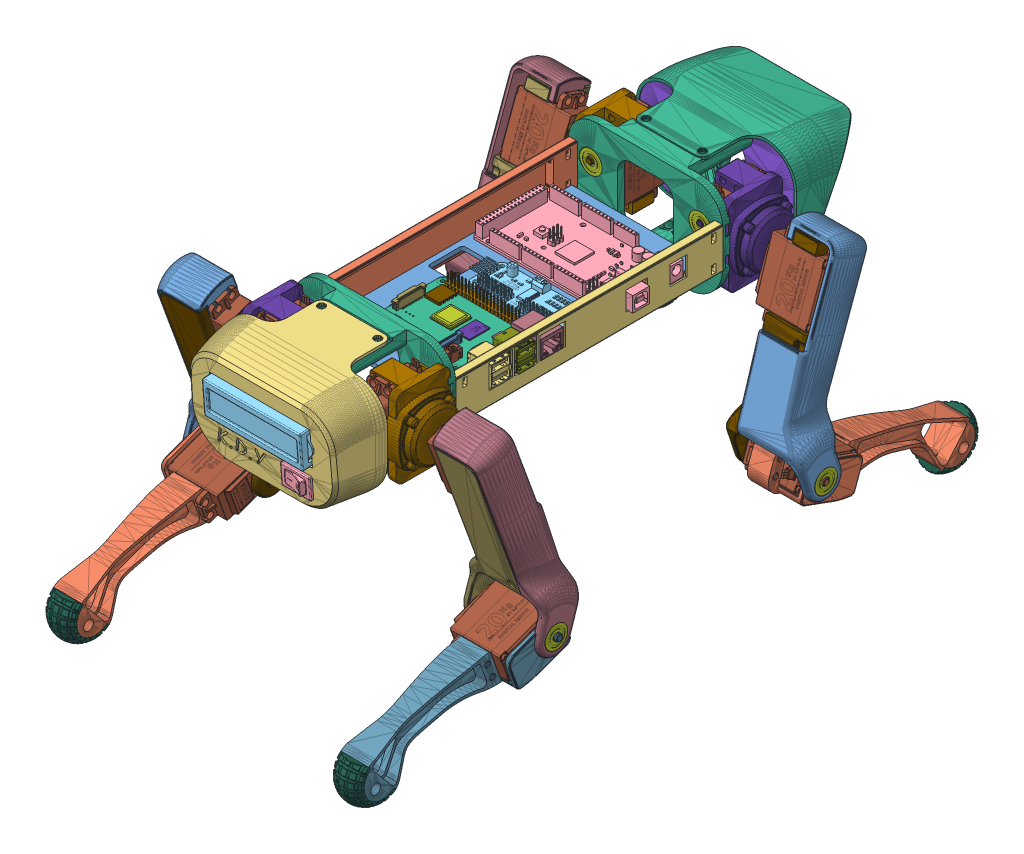
SolidWorks assembly Full Assembly [inverted legs], configuration Default. Lengths in mm.
Overall size (258.83 207.82 465.61).
182 component instances, 44 part files, 12 mates.
Components (placement in the parent):
- Chase Assembly-1: Chase Assembly [Default] at (121.4756 142.8431 224.0299) size (112.8 70 292)
  - 1_2MCU_Plate-1: 1_2MCU_Plate [Default] at (22.3647 94.0168 229.1495) size (106 5.81 180)
  - 2_2MCU_Left_side_plate-1: 2_2MCU_Left_side_plate [Default] at (18.1147 57.0168 99.1495) x (1 0 0) z (0 -1 0) size (6.5 190 29)
  - 3_2MCU_Right_side_plate-1: 3_2MCU_Right_side_plate [Default] at (121.6147 57.0168 169.1495) x (-1 0 0) z (0 -1 0) size (6.5 190 29)
  - ArduinoMega-1: ArduinoMega [Default] at (70.5126 101.4678 88.5891) x (1 0 0) z (0 -1 0) size (107.95 53.42 12.95)
  - _Hex_Screws-1: _Hex_Screws [H M3x8] at (55.5647 101.4678 97.3157) x (-0.837169 0 -0.546944) z (-0.546944 0 0.837169) size (5.5 10 6.35) (hidden)
  - _Hex_Screws-2: _Hex_Screws [H M3x8] at (55.5647 101.4678 69.2995) x (0.837169 0 0.546944) z (0.546944 0 -0.837169) size (5.5 10 6.35) (hidden)
  - 4_M3_nut-1: 4_M3_nut [Default] at (55.5655 95.0168 69.2614) x (0.855198 0 0.518302) z (-0.518302 0 0.855198) size (6 2.34 5.2) (hidden)
  - 4_M3_nut-2: 4_M3_nut [Default] at (55.5332 95.0168 97.2415) x (-0.878773 0 0.47724) z (-0.47724 0 -0.878773) size (6 2.34 5.2) (hidden)
  - 12Channel PWM-1: 12Channel PWM [Default] at (79.9147 99.8168 132.7995) x (0 0 -1) z (1 0 0) size (25.4 7.55 66.7)
  - _M2_nut-1: _M2_nut [Default] at (51.9456 95.5168 142.2881) x (-0.74075 0 -0.671781) z (0 -1 0) size (4.67 4.62 1.63) (hidden)
  - _M2_nut-2: _M2_nut [Default] at (107.8452 93.9168 142.288) x (-0.738205 0 -0.674577) z (0 1 0) size (4.67 4.62 1.63) (hidden)
  - _M2_nut-3: _M2_nut [Default] at (107.8453 93.9168 123.488) x (-0.739008 0 -0.673697) z (0 1 0) size (4.67 4.62 1.63) (hidden)
  - _M2_nut-4: _M2_nut [Default] at (51.8785 93.9168 123.4273) x (-0.741456 0 -0.671001) z (0 1 0) size (4.67 4.62 1.63) (hidden)
  - _Hex_Screws-3: _Hex_Screws [H M2x8] at (51.9647 101.3268 142.1995) x (0.837169 0 0.546944) z (0.546944 0 -0.837169) size (4 9.4 4.62) (hidden)
  - _Hex_Screws-4: _Hex_Screws [H M2x8] at (107.8647 101.3268 123.3995) x (0.837169 0 0.546944) z (0.546944 0 -0.837169) size (4 9.4 4.62) (hidden)
  - _Hex_Screws-5: _Hex_Screws [H M2x8] at (51.9647 101.3268 123.3995) x (0.837169 0 0.546944) z (0.546944 0 -0.837169) size (4 9.4 4.62) (hidden)
  - _Hex_Screws-6: _Hex_Screws [H M2x8] at (107.8647 101.3268 142.1995) x (0.837169 0 0.546944) z (0.546944 0 -0.837169) size (4 9.4 4.62) (hidden)
  - _Hex_Screws-11: _Hex_Screws [H M2x8] at (40.2647 101.4168 153.7995) x (0.837169 0 0.546944) z (0.546944 0 -0.837169) size (4 9.4 4.62) (hidden)
  - _Hex_Screws-12: _Hex_Screws [H M2x8] at (98.2647 101.4068 153.7995) x (0.837169 0 0.546944) z (0.546944 0 -0.837169) size (4 9.4 4.62) (hidden)
  - _Hex_Screws-13: _Hex_Screws [H M2x8] at (40.2647 101.4068 202.7995) x (0.837169 0 0.546944) z (0.546944 0 -0.837169) size (4 9.4 4.62) (hidden)
  - _Hex_Screws-14: _Hex_Screws [H M2x8] at (98.2647 101.4168 202.7995) x (0.837169 0 0.546944) z (0.546944 0 -0.837169) size (4 9.4 4.62) (hidden)
  - _M2_nut-9: _M2_nut [Default] at (98.2838 93.9168 153.7109) x (-0.741324 0 -0.671147) z (0 1 0) size (4.67 4.62 1.63) (hidden)
  - _M2_nut-10: _M2_nut [Default] at (40.2838 93.9168 202.711) x (-0.74083 0 -0.671693) z (0 1 0) size (4.67 4.62 1.63) (hidden)
  - _M2_nut-11: _M2_nut [Default] at (98.2457 93.9168 202.8881) x (-0.741502 0 -0.670951) z (0 1 0) size (4.67 4.62 1.63) (hidden)
  - _M2_nut-12: _M2_nut [Default] at (40.3319 95.5168 153.8603) x (-0.741456 0 -0.671001) z (0 -1 0) size (4.67 4.62 1.63) (hidden)
  - Raspberry Pi 4 Model B-1: Raspberry Pi 4 Model B [Default] at (79.2647 100.6168 178.2995) size (89 19.92 58.4)
    - Raspberry Pi 4 Model B.STEP-1: Raspberry Pi 4 Model B.STEP [Default] at origin size (89 19.92 58.4)
      - PCB, RPi4ModelB.STEP-1: PCB, RPi4ModelB.STEP [Default] at origin size (85 1.6 56)
      - Broadcom BCM2711B0 CPU, RPi4ModelB.STEP-1: Broadcom BCM2711B0 CPU, RPi4ModelB.STEP [Default] at (-13.25 0.8 -4.5) size (15 2.3 15)
      - 2.54 mm DUPONT MALE PIN HEADER, POE, 2X2, RPi4ModelB.STEP-1: 2.54 mm DUPONT MALE PIN HEADER, POE, 2X2, RPi4ModelB.STEP [Default] at (19 0.8 -18.36) size (5.08 11.3 5.08)
      - 2.54 mm DUPONT MALE PIN HEADER, IO, 2X20, RPi4ModelB.STEP-1: 2.54 mm DUPONT MALE PIN HEADER, IO, 2X20, RPi4ModelB.STEP [Default] at (-10 0.8 -24.5) size (50.8 11.3 5.08)
      - Camera Connector, RPi4ModelB.STEP-1: Camera Connector, RPi4ModelB.STEP [Default] at (4 0.8 16.5) x (0 0 -1) z (1 0 0) size (22.4 5.68 5.07)
      - Microphone Plug, RPi4ModelB.STEP-1: Microphone Plug, RPi4ModelB.STEP [Default] at (11.5 0.8 21.65) size (7.23 7.55 15)
      - Display Connector, RPi4ModelB.STEP-1: Display Connector, RPi4ModelB.STEP [Default] at (-38.5 0.8 0) x (0 0 1) z (-1 0 0) size (22.4 5.68 5.07)
      - Gigabit Ethernet Port, RPi4ModelB.STEP-1: Gigabit Ethernet Port, RPi4ModelB.STEP [Default] at (45.5 7.55 -17.75) x (0 0 -1) z (1 0 0) size (16.33 17.24 21.6)
      - Female Micro HDMI Connector, RPi4ModelB.STEP-1: Female Micro HDMI Connector, RPi4ModelB.STEP [Default] at (-3 0.8 27.3875) size (6.5 3.51 7.5)
      - Female Micro HDMI Connector, RPi4ModelB.STEP-2: Female Micro HDMI Connector, RPi4ModelB.STEP [Default] at (-16.5 0.8 27.3875) size (6.5 3.51 7.5)
      - Female USB Type C Connector, RPi4ModelB.STEP-1: Female USB Type C Connector, RPi4ModelB.STEP [Default] at (-31.3 0.8 26.5419) size (8.94 3.96 7.9)
      - 2X USB3.0 PORTS, RPi4ModelB.STEP-1: 2X USB3.0 PORTS, RPi4ModelB.STEP [Default] at (37.07 0.8 1) size (17.48 19.42 15.69)
      - 91D77 D9WHV 778K, 4 GB LPDDR4 SDRAM, RPi4ModelB.STEP-1: 91D77 D9WHV 778K, 4 GB LPDDR4 SDRAM, RPi4ModelB.STEP [Default] at (2.25 0.8 -4.5) size (10 0.8 14.5)
      - Cypress CYW43455 Wireless Module Cover, RPi4ModelB.STEP-1: Cypress CYW43455 Wireless Module Cover, RPi4ModelB.STEP [Default] at (-30.5 0.8 -14.5) size (11 1.6 13)
      - SD Card Slot, RPi4ModelB.STEP-1: SD Card Slot, RPi4ModelB.STEP [Default] at (-35.3 -0.8 0) x (0 0 -1) z (-1 0 0) size (11.95 1.45 11.4)
      - VIA VL805 PCIe USB 3.0 controller, RPi4ModelB.STEP-1: VIA VL805 PCIe USB 3.0 controller, RPi4ModelB.STEP [Default] at (17.5 0.8 4) size (8.8 0.8 8.8)
      - 2X USB2.0 PORTS, RPi4ModelB.STEP-1: 2X USB2.0 PORTS, RPi4ModelB.STEP [Default] at (37.065 0.65 19) size (17.87 19.17 15.35)
      - Broadcom BCM54213PE Gigabit Ethernet Transceiver, RPi4ModelB.STEP-1: Broadcom BCM54213PE Gigabit Ethernet Transceiver, RPi4ModelB.STEP [Default] at (16.5 0.8 -10) size (6.8 1 6.8)
      - MxL7704 Universal PMIC, RPi4ModelB.STEP-1: MxL7704 Universal PMIC, RPi4ModelB.STEP [Default] at (-32.5 0.8 16) size (5.4 0.8 5.4)
  - 6_Front_shoulder_mg-1: 6_Front_shoulder_mg [Default] at (124.8647 139.0168 39.1495) x (-1 0 0) z (0 -1 0) size (110 51 70)
  - 6_Front_shoulder_mg-2: 6_Front_shoulder_mg [Default] at (14.8647 139.0168 229.1495) x (1 0 0) z (0 -1 0) size (110 51 70)
  - _Hex_Screws-15: _Hex_Screws [H M3x12] at (18.2198 96.9886 231.1495) x (1 0 0) z (0 1 0) size (5.5 14 6.35) (hidden)
  - _Hex_Screws-16: _Hex_Screws [H M3x12] at (121.5159 97.0038 231.1495) x (1 0 0) z (0 1 0) size (5.5 14 6.35) (hidden)
  - _Hex_Screws-17: _Hex_Screws [H M3x12] at (18.2375 115.9459 231.1495) x (-0.998805 0.048869 0) z (-0.048869 -0.998805 0) size (5.5 14 6.35) (hidden)
  - _Hex_Screws-18: _Hex_Screws [H M3x12] at (18.1956 96.9701 37.1495) x (0.969974 0.243208 0) z (0.243208 -0.969974 0) size (5.5 14 6.35) (hidden)
  - _Hex_Screws-19: _Hex_Screws [H M3x12] at (18.1916 115.9399 37.1495) x (1 0 0) z (0 -1 0) size (5.5 14 6.35) (hidden)
  - _Hex_Screws-20: _Hex_Screws [H M3x12] at (121.5019 115.9701 231.1495) x (0.105991 0.994367 0) z (-0.994367 0.105991 0) size (5.5 14 6.35) (hidden)
  - _Hex_Screws-21: _Hex_Screws [H M3x12] at (121.6489 115.9342 37.1495) x (1 0 0) z (0 -1 0) size (5.5 14 6.35) (hidden)
  - _Hex_Screws-22: _Hex_Screws [H M3x12] at (121.6691 96.9226 37.1495) x (1 0 0) z (0 -1 0) size (5.5 14 6.35) (hidden)
  - 4_M3_nut-4: 4_M3_nut [Default] at (18.0647 96.9149 222.1495) x (1 0 0) z (0 -1 0) size (6 2.34 5.2) (hidden)
  - 4_M3_nut-5: 4_M3_nut [Default] at (18.0647 115.9149 222.1495) x (1 0 0) z (0 -1 0) size (6 2.34 5.2) (hidden)
  - 4_M3_nut-6: 4_M3_nut [Default] at (121.6647 96.9149 222.1495) x (1 0 0) z (0 -1 0) size (6 2.34 5.2) (hidden)
  - 4_M3_nut-7: 4_M3_nut [Default] at (121.6647 115.9149 222.1495) x (1 0 0) z (0 -1 0) size (6 2.34 5.2) (hidden)
  - 4_M3_nut-8: 4_M3_nut [Default] at (18.0647 115.9149 46.1495) x (0.5 0.866025 0) z (-0.866025 0.5 0) size (6 2.34 5.2) (hidden)
  - 4_M3_nut-9: 4_M3_nut [Default] at (18.0647 96.9149 44.1495) x (1 0 0) z (0 -1 0) size (6 2.34 5.2) (hidden)
  - 4_M3_nut-10: 4_M3_nut [Default] at (121.6647 96.9149 44.1495) x (1 0 0) z (0 -1 0) size (6 2.34 5.2) (hidden)
  - 4_M3_nut-11: 4_M3_nut [Default] at (121.6647 115.9149 46.1495) x (0.5 -0.866025 0) z (0.866025 0.5 0) size (6 2.34 5.2) (hidden)
  - F625ZZ Ball Bearing-1: F625ZZ Ball Bearing [Default] at (31.004 104.9515 234.1495) x (1 0 0) z (0 0 1) size (18 18 5)
  - F625ZZ Ball Bearing-2: F625ZZ Ball Bearing [Default] at (104.9018 120.0403 234.1495) x (-0.879341 -0.476193 0) z (0 0 1) size (18 18 5)
  - F625ZZ Ball Bearing-3: F625ZZ Ball Bearing [Default] at (30.2307 104.9537 34.1495) x (-0.995136 0.098516 0) z (0 0 -1) size (18 18 5)
  - F625ZZ Ball Bearing-4: F625ZZ Ball Bearing [Default] at (111.8008 105.7118 34.1495) x (-0.923728 -0.383049 0) z (0 0 -1) size (18 18 5)
- Front Legs-1: Front Legs [Default] at (233.7989 374.0539 299.7914) x (-1 0 0) z (0 -1 0) size (257.32 168.18 205.82)
  - 7_Rear_shoulder-2: 7_Rear_shoulder [Default] at (-12.5249 87.612 92.1876) size (110 5 66)
  - Left Leg Assembly-1: Left Leg Assembly [Default] at (86.5165 30.9423 148.2853) size (111.25 167.25 201.66)
    - Left_arm_joint_mg-1: Left_arm_joint_mg [Default] at (-15.0415 19.5698 -40.5977) size (37.5 46 56.5)
    - Servohorn-1: Servohorn [4 Prong] at (19.6585 29.8198 -20.3477) x (0 -0.698611 0.715501) z (-1 0 0) size (31.8 31.8 2.24)
    - Servo Motor-1: Servo Motor [Default] at (-5.0415 40.5698 -30.0977) size (20.1 45.99 55.6)
    - Servohorn-2: Servohorn [Default] at (-5.0415 60.9698 -30.0977) x (0.506689 0 -0.862129) z (0 -1 0) size (28.18 31.8 2.24)
    - Servo Motor-2: Servo Motor [Default] at (38.0585 29.8198 -20.3477) x (0 0.939693 0.34202) z (0 -0.34202 0.939693) size (20.1 45.99 55.6)
    - Left_arm_mg-1: Left_arm_mg [Default] at (38.0585 42.7737 -26.7003) x (0 -0.939693 -0.34202) z (0 -0.34202 0.939693) size (38.24 39.8 137.4)
    - SM_Left_arm_cover-1: SM_Left_arm_cover [Default] at (38.2585 50.3364 -32.5645) x (0 -0.939693 -0.34202) z (0 -0.34202 0.939693) size (41.16 45 143.55)
    - F625ZZ Ball Bearing-1: F625ZZ Ball Bearing [Default] at (78.2585 -1.6568 83.7617) x (0 -0.070361 0.997522) z (-1 0 0) size (18 18 5)
    - Servohorn-3: Servohorn [1 Prong] at (28.0585 6.3719 84.4796) x (0 0.893193 -0.449674) z (1 0 0) size (9.55 20.65 2.24)
    - Left_wrist_mg-1: Left_wrist_mg [Default] at (18.4585 0.3781 71.7095) x (0 0.939693 0.34202) z (0 -0.34202 0.939693) size (149.99 36.9 30)
    - foot-1: foot [Default] at (48.4585 115.3593 124.2008) x (0 0.642788 -0.766044) z (0 -0.766044 -0.642788) size (38.32 20 19.41)
    - Servo Motor-3: Servo Motor [Default] at (48.4585 6.3719 84.4796) x (0 0.34202 -0.939693) z (0 0.939693 0.34202) size (20.1 45.99 55.6)
    - _Hex_Screws-1: _Hex_Screws [H M4x20] at (-0.0415 43.7698 3.9023) x (-0.837169 0 -0.546944) z (-0.546944 0 0.837169) size (7 22.8 8.08) (hidden)
    - _Hex_Screws-2: _Hex_Screws [H M4x20] at (-10.0415 43.7698 -44.0977) x (-0.837169 0 -0.546944) z (-0.546944 0 0.837169) size (7 22.8 8.08) (hidden)
    - _Hex_Screws-3: _Hex_Screws [H M4x20] at (-10.0415 43.7698 3.9023) x (-0.837169 0 -0.546944) z (-0.546944 0 0.837169) size (7 22.8 8.08) (hidden)
    - _Hex_Screws-4: _Hex_Screws [H M4x20] at (-0.0415 43.7698 -44.0977) x (-0.837169 0 -0.546944) z (-0.546944 0 0.837169) size (7 22.8 8.08) (hidden)
    - _Hex_Screws-5: _Hex_Screws [H M4x20] at (34.8585 22.8895 13.3119) x (0 0.825172 -0.564882) z (0 -0.564882 -0.825172) size (7 22.8 8.08) (hidden)
    - _Hex_Screws-6: _Hex_Screws [H M4x20] at (34.8585 13.4926 9.8917) x (0 0.825172 -0.564882) z (0 -0.564882 -0.825172) size (7 22.8 8.08) (hidden)
    - _Hex_Screws-7: _Hex_Screws [H M4x20] at (34.8585 39.3065 -31.7933) x (0 0.802845 -0.596188) z (0 -0.596188 -0.802845) size (7 22.8 8.08) (hidden)
    - _Hex_Screws-8: _Hex_Screws [H M4x20] at (34.8585 29.9096 -35.2135) x (0 -0.944714 0.327896) z (0 0.327896 0.944714) size (7 22.8 8.08) (hidden)
    - _Hex_Screws-9: _Hex_Screws [H M4x20] at (45.2585 40.0315 91.4099) x (0 0.825172 -0.564882) z (0 -0.564882 -0.825172) size (7 22.8 8.08) (hidden)
    - _Hex_Screws-10: _Hex_Screws [H M4x20] at (45.2585 36.6113 100.8068) x (0 0.825172 -0.564882) z (0 -0.564882 -0.825172) size (7 22.8 8.08) (hidden)
    - _Hex_Screws-11: _Hex_Screws [H M4x20] at (45.2585 -5.0737 74.9929) x (0 0.825172 -0.564882) z (0 -0.564882 -0.825172) size (7 22.8 8.08) (hidden)
    - _Hex_Screws-12: _Hex_Screws [H M4x20] at (45.2585 -8.4939 84.3898) x (0 0.825172 -0.564882) z (0 -0.564882 -0.825172) size (7 22.8 8.08) (hidden)
    - _Hex_Screws-13: _Hex_Screws [H M3x16] at (62.9617 14.9879 55.4881) x (0.992954 0.04053 -0.111356) z (-0.118503 0.33961 -0.933071) size (5.5 18 6.35)
  - Right Leg Assembly-1: Right Leg Assembly [Default] at (19.1728 32.9715 132.7261) size (98.95 167.45 200.32)
    - Right_arm_joint_mg-1: Right_arm_joint_mg [Default] at (24.2858 18.5405 -25.0321) size (37.5 46 56.5)
    - Servohorn-1: Servohorn [4 Prong] at (-38.4142 28.7905 -4.7821) x (0 0.715501 0.698611) z (-1 0 0) size (31.8 31.8 2.24)
    - Servo Motor-1: Servo Motor [Default] at (-15.7142 38.5405 -14.5321) size (20.1 45.99 55.6)
    - Servohorn-2: Servohorn [Default] at (-15.7142 58.9405 -14.5321) x (-0.99999 0 0.00451) z (0 -1 0) size (28.18 31.8 2.24)
    - Right_arm_mg-1: Right_arm_mg [Default] at (-8.8142 41.6076 -10.7588) x (0 -0.939693 -0.34202) z (0 -0.34202 0.939693) size (38.24 39.8 137.4)
    - SM_Right_arm_cover-1: SM_Right_arm_cover [Default] at (-48.6142 49.0427 -16.5661) x (0 -0.939693 -0.34202) z (0 -0.34202 0.939693) size (41.16 45 143.55)
    - F625ZZ Ball Bearing-1: F625ZZ Ball Bearing [Default] at (-98.6142 -2.6723 100.0196) x (0 0.0383 -0.999266) z (1 0 0) size (18 18 5)
    - Servohorn-3: Servohorn [1 Prong] at (-48.8142 5.2058 100.4211) x (0 -0.953491 0.301422) z (-1 0 0) size (9.55 20.65 2.24)
    - Servo Motor-2: Servo Motor [Default] at (-67.7142 5.2058 100.4211) x (0 -0.34202 0.939693) z (0 0.939693 0.34202) size (20.1 45.99 55.6)
    - Servo Motor-3: Servo Motor [Default] at (-58.8142 28.7905 -4.7821) x (0 -0.939693 -0.34202) z (0 -0.34202 0.939693) size (20.1 45.99 55.6)
    - Right_wrist_mg-1: Right_wrist_mg [Default] at (-67.7142 -0.7709 87.604) x (0 0.939693 0.34202) z (0 -0.34202 0.939693) size (149.99 36.9 30)
    - foot-1: foot [Default] at (-67.7142 114.2242 140.0873) x (0 -0.656061 0.754708) z (0 -0.754708 -0.656061) size (38.32 20 19.41)
    - _Hex_Screws-1: _Hex_Screws [H M4x20] at (-20.7142 41.7405 19.4679) x (-0.837169 0 -0.546944) z (-0.546944 0 0.837169) size (7 22.8 8.08) (hidden)
    - _Hex_Screws-2: _Hex_Screws [H M4x20] at (-10.7142 41.7405 -28.5321) x (-0.837169 0 -0.546944) z (-0.546944 0 0.837169) size (7 22.8 8.08) (hidden)
    - _Hex_Screws-3: _Hex_Screws [H M4x20] at (-10.7142 41.7405 19.4679) x (-0.99108 0 -0.133267) z (-0.133267 0 0.99108) size (7 22.8 8.08) (hidden)
    - _Hex_Screws-4: _Hex_Screws [H M4x20] at (-20.7142 41.7405 -28.5321) x (0.837169 0 0.546944) z (0.546944 0 -0.837169) size (7 22.8 8.08) (hidden)
    - _Hex_Screws-5: _Hex_Screws [H M4x20] at (-55.6142 28.8803 -19.6479) x (0 0.085299 -0.996355) z (0 0.996355 0.085299) size (7 22.8 8.08) (hidden)
    - _Hex_Screws-8: _Hex_Screws [H M4x20] at (-55.6142 12.4633 25.4573) x (0 -0.381849 0.924225) z (0 -0.924225 -0.381849) size (7 22.8 8.08) (hidden)
    - _Hex_Screws-9: _Hex_Screws [H M4x20] at (-55.6142 21.8603 28.8775) x (0 -0.381849 0.924225) z (0 -0.924225 -0.381849) size (7 22.8 8.08) (hidden)
    - _Hex_Screws-10: _Hex_Screws [H M4x20] at (-64.5142 -9.66 100.3313) x (0 -0.381849 0.924225) z (0 -0.924225 -0.381849) size (7 22.8 8.08) (hidden)
    - _Hex_Screws-11: _Hex_Screws [H M4x20] at (-64.5142 38.8655 107.3514) x (0 -0.381849 0.924225) z (0 -0.924225 -0.381849) size (7 22.8 8.08) (hidden)
    - _Hex_Screws-12: _Hex_Screws [H M4x20] at (-64.5142 -6.2398 90.9344) x (0 -0.381849 0.924225) z (0 -0.924225 -0.381849) size (7 22.8 8.08) (hidden)
    - _Hex_Screws-14: _Hex_Screws [H M4x20] at (-64.5142 35.4453 116.7483) x (0 -0.381849 0.924225) z (0 -0.924225 -0.381849) size (7 22.8 8.08) (hidden)
    - _Hex_Screws-15: _Hex_Screws [H M4x20] at (-55.6142 38.2772 -16.2277) x (0 0.381849 -0.924225) z (0 0.924225 0.381849) size (7 22.8 8.08) (hidden)
    - _Hex_Screws-19: _Hex_Screws [H M3x16] at (-83.8911 13.8209 71.432) x (0.19625 0.335369 -0.921419) z (-0.980554 0.067122 -0.184415) size (5.5 18 6.35)
- Front Legs-2: Front Legs [Default] at (148.8817 374.0539 416.5673) x (1 0 0) z (0 -1 0) size (257.32 168.18 205.82)
  - 7_Rear_shoulder-2: 7_Rear_shoulder [Default] at (-12.5249 87.612 92.1876) size (110 5 66)
  - Left Leg Assembly-1: Left Leg Assembly [Default] at (86.5165 30.9423 148.2853) size (111.25 167.25 201.66)
    - Left_arm_joint_mg-1: Left_arm_joint_mg [Default] at (-15.0415 19.5698 -40.5977) size (37.5 46 56.5)
    - Servohorn-1: Servohorn [4 Prong] at (19.6585 29.8198 -20.3477) x (0 -0.698611 0.715501) z (-1 0 0) size (31.8 31.8 2.24)
    - Servo Motor-1: Servo Motor [Default] at (-5.0415 40.5698 -30.0977) size (20.1 45.99 55.6)
    - Servohorn-2: Servohorn [Default] at (-5.0415 60.9698 -30.0977) x (0.506689 0 -0.862129) z (0 -1 0) size (28.18 31.8 2.24)
    - Servo Motor-2: Servo Motor [Default] at (38.0585 29.8198 -20.3477) x (0 0.939693 0.34202) z (0 -0.34202 0.939693) size (20.1 45.99 55.6)
    - Left_arm_mg-1: Left_arm_mg [Default] at (38.0585 42.7737 -26.7003) x (0 -0.939693 -0.34202) z (0 -0.34202 0.939693) size (38.24 39.8 137.4)
    - SM_Left_arm_cover-1: SM_Left_arm_cover [Default] at (38.2585 50.3364 -32.5645) x (0 -0.939693 -0.34202) z (0 -0.34202 0.939693) size (41.16 45 143.55)
    - F625ZZ Ball Bearing-1: F625ZZ Ball Bearing [Default] at (78.2585 -1.6568 83.7617) x (0 -0.070361 0.997522) z (-1 0 0) size (18 18 5)
    - Servohorn-3: Servohorn [1 Prong] at (28.0585 6.3719 84.4796) x (0 0.893193 -0.449674) z (1 0 0) size (9.55 20.65 2.24)
    - Left_wrist_mg-1: Left_wrist_mg [Default] at (18.4585 0.3781 71.7095) x (0 0.939693 0.34202) z (0 -0.34202 0.939693) size (149.99 36.9 30)
    - foot-1: foot [Default] at (48.4585 115.3593 124.2008) x (0 0.642788 -0.766044) z (0 -0.766044 -0.642788) size (38.32 20 19.41)
    - Servo Motor-3: Servo Motor [Default] at (48.4585 6.3719 84.4796) x (0 0.34202 -0.939693) z (0 0.939693 0.34202) size (20.1 45.99 55.6)
    - _Hex_Screws-1: _Hex_Screws [H M4x20] at (-0.0415 43.7698 3.9023) x (-0.837169 0 -0.546944) z (-0.546944 0 0.837169) size (7 22.8 8.08) (hidden)
    - _Hex_Screws-2: _Hex_Screws [H M4x20] at (-10.0415 43.7698 -44.0977) x (-0.837169 0 -0.546944) z (-0.546944 0 0.837169) size (7 22.8 8.08) (hidden)
    - _Hex_Screws-3: _Hex_Screws [H M4x20] at (-10.0415 43.7698 3.9023) x (-0.837169 0 -0.546944) z (-0.546944 0 0.837169) size (7 22.8 8.08) (hidden)
    - _Hex_Screws-4: _Hex_Screws [H M4x20] at (-0.0415 43.7698 -44.0977) x (-0.837169 0 -0.546944) z (-0.546944 0 0.837169) size (7 22.8 8.08) (hidden)
    - _Hex_Screws-5: _Hex_Screws [H M4x20] at (34.8585 22.8895 13.3119) x (0 0.825172 -0.564882) z (0 -0.564882 -0.825172) size (7 22.8 8.08) (hidden)
    - _Hex_Screws-6: _Hex_Screws [H M4x20] at (34.8585 13.4926 9.8917) x (0 0.825172 -0.564882) z (0 -0.564882 -0.825172) size (7 22.8 8.08) (hidden)
    - _Hex_Screws-7: _Hex_Screws [H M4x20] at (34.8585 39.3065 -31.7933) x (0 0.802845 -0.596188) z (0 -0.596188 -0.802845) size (7 22.8 8.08) (hidden)
    - _Hex_Screws-8: _Hex_Screws [H M4x20] at (34.8585 29.9096 -35.2135) x (0 -0.944714 0.327896) z (0 0.327896 0.944714) size (7 22.8 8.08) (hidden)
    - _Hex_Screws-9: _Hex_Screws [H M4x20] at (45.2585 40.0315 91.4099) x (0 0.825172 -0.564882) z (0 -0.564882 -0.825172) size (7 22.8 8.08) (hidden)
    - _Hex_Screws-10: _Hex_Screws [H M4x20] at (45.2585 36.6113 100.8068) x (0 0.825172 -0.564882) z (0 -0.564882 -0.825172) size (7 22.8 8.08) (hidden)
    - _Hex_Screws-11: _Hex_Screws [H M4x20] at (45.2585 -5.0737 74.9929) x (0 0.825172 -0.564882) z (0 -0.564882 -0.825172) size (7 22.8 8.08) (hidden)
    - _Hex_Screws-12: _Hex_Screws [H M4x20] at (45.2585 -8.4939 84.3898) x (0 0.825172 -0.564882) z (0 -0.564882 -0.825172) size (7 22.8 8.08) (hidden)
    - _Hex_Screws-13: _Hex_Screws [H M3x16] at (62.9617 14.9879 55.4881) x (0.992954 0.04053 -0.111356) z (-0.118503 0.33961 -0.933071) size (5.5 18 6.35)
  - Right Leg Assembly-1: Right Leg Assembly [Default] at (19.1728 32.9715 132.7261) size (98.95 167.45 200.32)
    - Right_arm_joint_mg-1: Right_arm_joint_mg [Default] at (24.2858 18.5405 -25.0321) size (37.5 46 56.5)
    - Servohorn-1: Servohorn [4 Prong] at (-38.4142 28.7905 -4.7821) x (0 0.715501 0.698611) z (-1 0 0) size (31.8 31.8 2.24)
    - Servo Motor-1: Servo Motor [Default] at (-15.7142 38.5405 -14.5321) size (20.1 45.99 55.6)
    - Servohorn-2: Servohorn [Default] at (-15.7142 58.9405 -14.5321) x (-0.99999 0 0.00451) z (0 -1 0) size (28.18 31.8 2.24)
    - Right_arm_mg-1: Right_arm_mg [Default] at (-8.8142 41.6076 -10.7588) x (0 -0.939693 -0.34202) z (0 -0.34202 0.939693) size (38.24 39.8 137.4)
    - SM_Right_arm_cover-1: SM_Right_arm_cover [Default] at (-48.6142 49.0427 -16.5661) x (0 -0.939693 -0.34202) z (0 -0.34202 0.939693) size (41.16 45 143.55)
    - F625ZZ Ball Bearing-1: F625ZZ Ball Bearing [Default] at (-98.6142 -2.6723 100.0196) x (0 0.0383 -0.999266) z (1 0 0) size (18 18 5)
    - Servohorn-3: Servohorn [1 Prong] at (-48.8142 5.2058 100.4211) x (0 -0.953491 0.301422) z (-1 0 0) size (9.55 20.65 2.24)
    - Servo Motor-2: Servo Motor [Default] at (-67.7142 5.2058 100.4211) x (0 -0.34202 0.939693) z (0 0.939693 0.34202) size (20.1 45.99 55.6)
    - Servo Motor-3: Servo Motor [Default] at (-58.8142 28.7905 -4.7821) x (0 -0.939693 -0.34202) z (0 -0.34202 0.939693) size (20.1 45.99 55.6)
    - Right_wrist_mg-1: Right_wrist_mg [Default] at (-67.7142 -0.7709 87.604) x (0 0.939693 0.34202) z (0 -0.34202 0.939693) size (149.99 36.9 30)
    - foot-1: foot [Default] at (-67.7142 114.2242 140.0873) x (0 -0.656061 0.754708) z (0 -0.754708 -0.656061) size (38.32 20 19.41)
    - _Hex_Screws-1: _Hex_Screws [H M4x20] at (-20.7142 41.7405 19.4679) x (-0.837169 0 -0.546944) z (-0.546944 0 0.837169) size (7 22.8 8.08) (hidden)
    - _Hex_Screws-2: _Hex_Screws [H M4x20] at (-10.7142 41.7405 -28.5321) x (-0.837169 0 -0.546944) z (-0.546944 0 0.837169) size (7 22.8 8.08) (hidden)
    - _Hex_Screws-3: _Hex_Screws [H M4x20] at (-10.7142 41.7405 19.4679) x (-0.99108 0 -0.133267) z (-0.133267 0 0.99108) size (7 22.8 8.08) (hidden)
    - _Hex_Screws-4: _Hex_Screws [H M4x20] at (-20.7142 41.7405 -28.5321) x (0.837169 0 0.546944) z (0.546944 0 -0.837169) size (7 22.8 8.08) (hidden)
    - _Hex_Screws-5: _Hex_Screws [H M4x20] at (-55.6142 28.8803 -19.6479) x (0 0.085299 -0.996355) z (0 0.996355 0.085299) size (7 22.8 8.08) (hidden)
    - _Hex_Screws-8: _Hex_Screws [H M4x20] at (-55.6142 12.4633 25.4573) x (0 -0.381849 0.924225) z (0 -0.924225 -0.381849) size (7 22.8 8.08) (hidden)
    - _Hex_Screws-9: _Hex_Screws [H M4x20] at (-55.6142 21.8603 28.8775) x (0 -0.381849 0.924225) z (0 -0.924225 -0.381849) size (7 22.8 8.08) (hidden)
    - _Hex_Screws-10: _Hex_Screws [H M4x20] at (-64.5142 -9.66 100.3313) x (0 -0.381849 0.924225) z (0 -0.924225 -0.381849) size (7 22.8 8.08) (hidden)
    - _Hex_Screws-11: _Hex_Screws [H M4x20] at (-64.5142 38.8655 107.3514) x (0 -0.381849 0.924225) z (0 -0.924225 -0.381849) size (7 22.8 8.08) (hidden)
    - _Hex_Screws-12: _Hex_Screws [H M4x20] at (-64.5142 -6.2398 90.9344) x (0 -0.381849 0.924225) z (0 -0.924225 -0.381849) size (7 22.8 8.08) (hidden)
    - _Hex_Screws-14: _Hex_Screws [H M4x20] at (-64.5142 35.4453 116.7483) x (0 -0.381849 0.924225) z (0 -0.924225 -0.381849) size (7 22.8 8.08) (hidden)
    - _Hex_Screws-15: _Hex_Screws [H M4x20] at (-55.6142 38.2772 -16.2277) x (0 0.381849 -0.924225) z (0 0.924225 0.381849) size (7 22.8 8.08) (hidden)
    - _Hex_Screws-19: _Hex_Screws [H M3x16] at (-83.8911 13.8209 71.432) x (0.19625 0.335369 -0.921419) z (-0.980554 0.067122 -0.184415) size (5.5 18 6.35)
- Back Assembly-1: Back Assembly [Default] at (224.5857 241.5151 483.7838) x (0 -1 0) z (0 0 -1) size (70 114 75.42)
  - SM_Rear_cover_mg-1: SM_Rear_cover_mg [Default] at (-38.2447 -23.7546 -24.8955) size (70 114 69.85)
  - rocker switch 1-1: rocker switch 1 [test] at (14.374 8.6954 -53.0846) x (-0.997054 0 -0.076697) z (0.076697 0 -0.997054) size (15 21 21.16)
  - LCDScreen-1: LCDScreen [Default] at (-11.6228 33.6204 -49.4804) x (0 -1 0) z (0.997054 0 0.076697) size (79.38 18.26 34.92)
- SM_Front_cover_mg-1: SM_Front_cover_mg [Default] at (134.3403 281.7599 237.6794) x (0 0 -1) z (0 -1 0) size (92.81 114 70)
Mates (geometry in assembly coordinates):
- Concentric2: concentric: circle of Chase Assembly-1/6_Front_shoulder_mg-2; circle of Front Legs-1/7_Rear_shoulder-2
- Parallel1: parallel: plane of Chase Assembly-1/6_Front_shoulder_mg-2 through (136.3403 279.8599 453.1794) normal (0 1 0); plane of Front Legs-1/7_Rear_shoulder-2 through (246.3238 279.8663 546.7456) normal (0 1 0)
- Concentric5: concentric: circle of Chase Assembly-1/6_Front_shoulder_mg-1; circle of Front Legs-2/7_Rear_shoulder-2
- Parallel2: parallel: plane of Chase Assembly-1/6_Front_shoulder_mg-1 through (246.3403 279.8599 263.1794) normal (0 1 0); plane of Front Legs-2/7_Rear_shoulder-2 through (136.3568 279.8663 163.307) normal (0 1 0)
- Coincident14: coincident anti-aligned: plane of Chase Assembly-1/6_Front_shoulder_mg-2 through (136.3403 279.8599 453.1794) normal (0 1 0); plane of Back Assembly-1/SM_Rear_cover_mg-1 through (248.3403 279.8599 508.6794) normal (0 -1 0)
- Distance1: distance = 1 mm anti-aligned: plane of Chase Assembly-1/6_Front_shoulder_mg-2 through (136.3403 281.8599 467.6794) normal (0 0 1); plane of Back Assembly-1/SM_Rear_cover_mg-1 through (248.3403 279.7599 468.6794) normal (0 0 -1)
- Coincident16: coincident aligned: plane of Chase Assembly-1/6_Front_shoulder_mg-2 through (216.3403 281.8599 453.1794) normal (1 0 0); plane of Back Assembly-1/SM_Rear_cover_mg-1 through (216.3403 279.7599 508.6794) normal (1 0 0)
- Coincident17: coincident anti-aligned: plane of Chase Assembly-1/6_Front_shoulder_mg-1 through (246.3403 279.8599 263.1794) normal (0 1 0); plane of SM_Front_cover_mg-1 through (134.3403 279.8599 237.6794) normal (0 -1 0)
- Coincident19: coincident aligned: plane of Chase Assembly-1/6_Front_shoulder_mg-1 through (166.3403 281.8599 263.1794) normal (-1 0 0); plane of SM_Front_cover_mg-1 through (166.3403 281.7599 237.6794) normal (-1 0 0)
- Distance2: distance = 1 mm anti-aligned: plane of SM_Front_cover_mg-1 through (134.3403 281.7599 247.6794) normal (0 0 1); plane of Chase Assembly-1/6_Front_shoulder_mg-1 through (246.3403 281.8599 248.6794) normal (0 0 -1)
- Coincident20: coincident: line of Chase Assembly-1/6_Front_shoulder_mg-2 through (172.8858 275.274 504.1794) axis (0.999937 -0.011236 0); plane of Front Legs-2/7_Rear_shoulder-2 through (136.3568 281.8663 504.1794) normal (0 0 -1)
- Coincident21: coincident: line of Chase Assembly-1/6_Front_shoulder_mg-1 through (209.7948 274.4458 212.1794) axis (-1 0 0); plane of Front Legs-1/7_Rear_shoulder-2 through (246.3238 281.8663 212.1794) normal (0 0 1)
